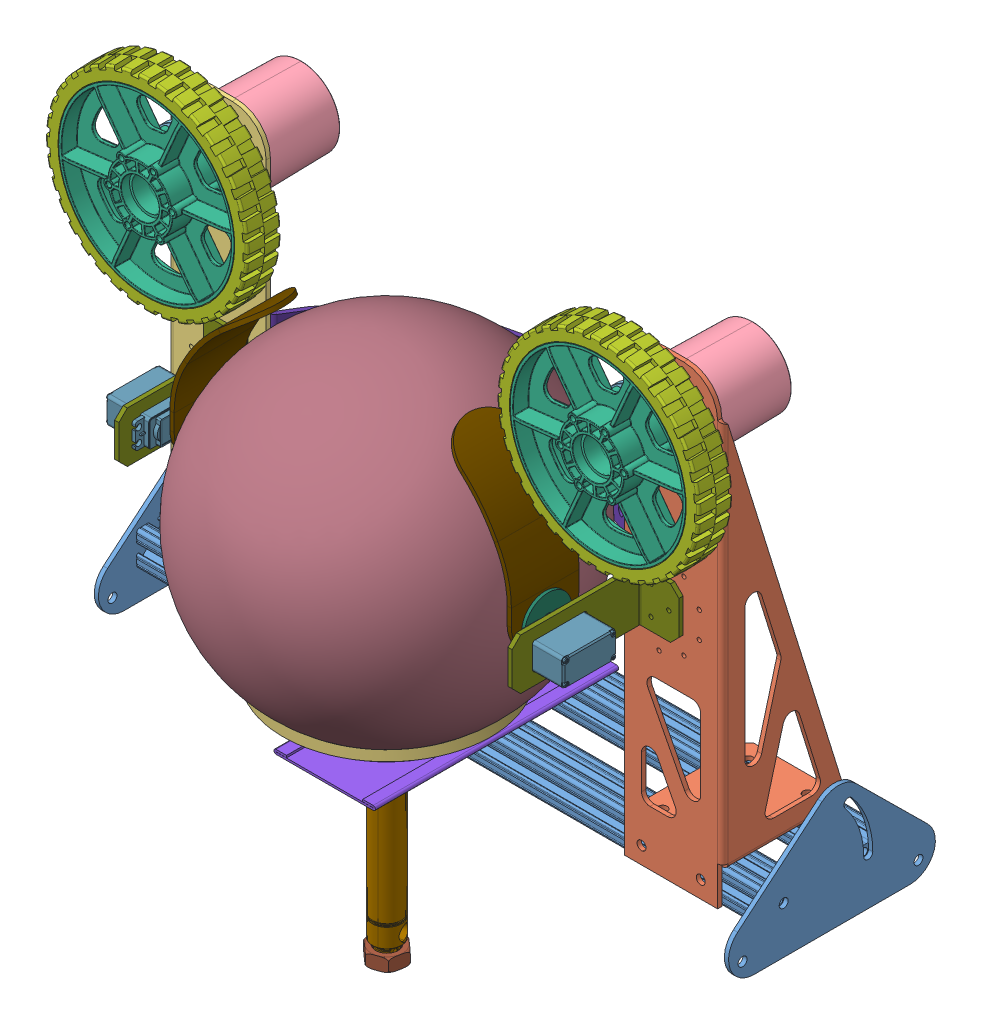
SolidWorks assembly Shooter, configuration Default. Lengths in mm.
Overall size (530.15 526.46 390.38).
32 component instances, 19 part files, 80 mates.
Components (placement in the parent):
- Shooter Base-1: Shooter Base [Default<As Machined>] at (0 35.306 -74.6762) size (469.9 25.4 88.9)
- Shooter Arm Right-1: Shooter Arm Right [Default] at (-100.3808 22.606 -61.9762) x (-1 0 0) z (0 0 -1) size (73.76 342.9 92.82)
- Shooter Arm-2: Shooter Arm [Default] at (-439.3692 22.606 -61.9762) x (-1 0 0) z (0 0 -1) size (73.76 342.9 92.82)
- REV-21-1650-1: REV-21-1650 [Default] at (-404.4442 327.406 -61.9762) x (0 1 0) z (0 0 1) size (61.14 61.02 93.25)
- REV-21-1650-2: REV-21-1650 [Default] at (-65.4558 327.406 -61.9762) x (0 1 0) z (0 0 1) size (61.14 61.02 93.25)
- am-0320a 8mm Key Hub.step-1: am-0320a 8mm Key Hub.step [Default] at (-404.4442 327.406 -33.0762) x (0.116635 -0.993175 0) z (0 0 -1) size (57.15 57.15 25.4)
- am-0320a 8mm Key Hub.step-2: am-0320a 8mm Key Hub.step [Default] at (-65.4558 327.406 -33.0762) x (0.114086 -0.993471 0) z (0 0 -1) size (57.15 57.15 25.4)
- am-0940b 6 in HiGrip Wheel-1: am-0940b 6 in HiGrip Wheel [Default] at (-424.5772 315.5538 -69.1474) x (0 0 -1) z (0.993175 0.116635 0) size (34.94 152.4 152.4)
  - 6 wheel Rev 4-1: 6 wheel Rev 4 [Default] at (-52.6446 9.4231 21.378) size (34.94 132.08 132.08)
  - 6 wheel tread II-1: 6 wheel tread II [Default] at (-65.3446 9.4231 21.378) x (0 0 -1) z (1 0 0) size (152.4 152.4 25.61)
- am-0940b 6 in HiGrip Wheel-2: am-0940b 6 in HiGrip Wheel [Default] at (-85.757 338.9677 -69.1474) x (0 0 -1) z (0.595537 -0.803328 0) size (34.94 152.4 152.4)
  - 6 wheel Rev 4-1: 6 wheel Rev 4 [Default] at (-52.6446 9.4231 21.378) size (34.94 132.08 132.08)
  - 6 wheel tread II-1: 6 wheel tread II [Default] at (-65.3446 9.4231 21.378) x (0 0 -1) z (1 0 0) size (152.4 152.4 25.61)
- Shooter Pneumatic Plate-1: Shooter Pneumatic Plate [Default] at (-196.85 49.5935 31.866) size (76.2 3.28 182.74)
- am-2034_2-1: am-2034_2 [Default] at (-234.95 -22.225 -14.9298) x (0.323379 0 0.94627) z (0 1 0) size (27.58 27.58 165.86) (flexible)
  - NCME075-0200.step_NCM-Body_075E^am-2034_2-1: NCME075-0200.step_NCM-Body_075E^am-2034_2 [Default] at origin size (21.84 21.85 153.16) (virtual)
  - NCME075-0200.step_NCM-Rod_075^am-2034_2-1: NCME075-0200.step_NCM-Rod_075^am-2034_2 [Default] at (0 0 -25.4) x (-1 0 0) z (0 0 1) size (19.05 19.05 123.53) (virtual)
  - NCME075-0200.step_NCM-Nut_075^am-2034_2-1: NCME075-0200.step_NCM-Nut_075^am-2034_2 [Default] at (0 0 77.439) x (-1 0 0) z (0 0 1) size (27.58 27.58 9.66) (virtual)
  - NCME075-0200.step_NCM-Nut_075^am-2034_2-2: NCME075-0200.step_NCM-Nut_075^am-2034_2 [Default] at (0 0 -63.119) size (27.58 27.58 9.66) (virtual)
- Shooter Cup-1: Shooter Cup [Default] at (-234.95 60.706 -14.9298) x (0.902068 0 -0.431594) z (0.431594 0 0.902068) size (155.9 37.46 155.9)
- Blue Cargo-1: Blue Cargo [Default] at (-234.95 193.4194 -14.9298) x (0.867373 -0.45742 -0.196039) z (0.420003 0.461532 0.7814) size (241.3 241.3 241.3)
- Hitec HS-325HB Korpus-3: Hitec HS-325HB Korpus [По умолчанию] at (-407.5 199.992 3.8708) x (0 0 1) z (0 1 0) size (53 41.52 20)
- Hitec HS-325HB Korpus-5: Hitec HS-325HB Korpus [По умолчанию] at (-62.4 200.82 5.0188) x (0 0 1) z (0 -1 0) size (53 41.52 20)
- Servo Horn Round-1: Servo Horn Round [Default] at (-369.3782 199.992 -6.1292) x (0 0.662146 0.749375) z (0 0.749375 -0.662146) size (35.33 5.66 35.33)
- Servo Horn Round-2: Servo Horn Round [Default] at (-100.5218 200.82 -4.9812) x (0 -0.231211 -0.972904) z (0 0.972904 -0.231211) size (35.33 5.66 35.33)
- Shooter Servo Mount-1: Shooter Servo Mount [Default] at (-84.9884 181.356 -55.6262) size (32.49 38.1 99.06)
- Shooter Servo Mount-2: Shooter Servo Mount [Default] at (-384.9116 219.456 -55.6262) x (-1 0 0) z (0 0 1) size (32.49 38.1 99.06)
- Shooter Back-1: Shooter Back [Default] at (-234.95 200.406 -65.1512) x (1 0 0) z (0 -1 0) size (403.96 84.05 76.2)
- Shooter Holders 2-1: Shooter Holders 2 [Default] at (-363.714 180.942 -31.5292) x (0 -1 0) z (0 0 1) size (125.91 60.15 53.7)
- Shooter Holders 2-2: Shooter Holders 2 [Default] at (-106.186 181.77 20.4188) x (0 -1 0) z (0 0 -1) size (125.91 60.15 53.7)
- Shooter Mount-1: Shooter Mount [Default] at (3.175 0 0) x (0 0 -1) z (1 0 0) size (215.9 98 3.17)
- Shooter Mount-2: Shooter Mount [Default] at (-469.9 0 0) x (0 0 -1) z (1 0 0) size (215.9 98 3.17)
Mates (geometry in assembly coordinates):
- Coincident7: coincident anti-aligned: plane of Shooter Base-1 through (-469.9 41.6391 -61.9762) normal (0 0 1); plane of Shooter Arm-2 through (-413.9692 340.106 -61.9762) normal (0 0 -1)
- Coincident9: coincident anti-aligned: plane of Shooter Base-1 through (-469.9 48.006 -81.0094) normal (0 1 0); plane of Shooter Arm-2 through (-439.3692 48.006 -61.9762) normal (0 -1 0)
- Coincident10: coincident anti-aligned: plane of Shooter Base-1 through (-469.9 48.006 -65.1258) normal (0 1 0); plane of Shooter Arm Right-1 through (-100.3808 48.006 -61.9762) normal (0 -1 0)
- Coincident11: coincident anti-aligned: plane of Shooter Base-1 through (-469.9 41.6391 -61.9762) normal (0 0 1); plane of Shooter Arm Right-1 through (-74.9808 340.106 -61.9762) normal (0 0 -1)
- Concentric1: concentric: cylinder of Shooter Arm-2 through (-404.4442 327.406 -58.8012) axis (0 0 -1) radius 9.0488; cylinder of Sport Planetary Gear Box-1/am-XXXX - 57 Sport 500 Hex Output Plug-1/Output Block-1 through (-279.4 242.0366 15.875) axis (0 0 -1) radius 19.05
- Coincident13: coincident: plane of Shooter Arm-2 through (-304.8 16.6116 9.525) normal (0 0 -1); plane of Sport Planetary Gear Box-1/am-XXXX - 57 Sport 500 Hex Output Plug-1/Output Block-1 through (-279.4 242.0366 9.525) normal (0 0 1)
- Parallel1: parallel aligned: plane of Shooter Arm-2 through (-413.9692 365.506 -58.8012) normal (0 1 0); plane of Sport Planetary Gear Box-1/am-XXXX - 57 Sport 1 Stage Ring Gear Housing-1 through (-303.2125 265.8491 6.35) normal (0 1 0)
- Concentric2: concentric aligned: cylinder of Shooter Arm-2 through (-404.4442 327.406 -58.8012) axis (0 0 -1) radius 9.0488; cylinder of REV-21-1650-1 through (-404.4442 327.406 -58.4762) axis (0 0 -1) radius 9.525
- Coincident15: coincident anti-aligned: plane of Shooter Arm-2 through (-413.9692 340.106 -61.9762) normal (0 0 -1); plane of REV-21-1650-1 through (-404.4442 327.406 -61.9762) normal (0 0 1)
- Parallel12: parallel aligned: plane of REV-21-1650-1 through (-404.4442 327.406 -61.9762) normal (-1 0 0); plane of Shooter Arm-2 through (-443.2808 22.606 -61.9762) normal (-1 0 0)
- Concentric3: concentric aligned: cylinder of Shooter Arm Right-1 through (-65.4558 327.406 -58.8012) axis (0 0 -1) radius 9.0488; cylinder of REV-21-1650-2 through (-65.4558 327.406 -58.4762) axis (0 0 -1) radius 9.525
- Coincident23: coincident anti-aligned: plane of Shooter Arm Right-1 through (-74.9808 340.106 -61.9762) normal (0 0 -1); plane of REV-21-1650-2 through (-65.4558 327.406 -61.9762) normal (0 0 1)
- Parallel13: parallel aligned: plane of Shooter Arm Right-1 through (-100.3808 22.606 -58.8012) normal (-1 0 0); plane of REV-21-1650-2 through (-65.4558 327.406 -61.9762) normal (-1 0 0)
- Concentric5: concentric aligned: cylinder of REV-21-1650-1 through (-404.4442 327.406 19.3375) axis (0 0 -1) radius 4; cylinder of am-0320a 8mm Key Hub.step-1 through (-404.4442 327.406 -33.0762) axis (0 0 -1) radius 4.0259
- Concentric6: concentric aligned: cylinder of REV-21-1650-2 through (-65.4558 327.406 19.3375) axis (0 0 -1) radius 4; cylinder of am-0320a 8mm Key Hub.step-2 through (-65.4558 327.406 -33.0762) axis (0 0 -1) radius 4.0259
- Concentric7: concentric anti-aligned: cylinder of REV-21-1650-1 through (-404.4442 327.406 19.3375) axis (0 0 -1) radius 4; cone of am-0940b 6 in HiGrip Wheel-1/6 wheel Rev 4-1 through (-404.4442 327.406 -16.5027) axis (0 0 1)
- Coincident25: coincident anti-aligned: plane of am-0320a 8mm Key Hub.step-1 through (-411.6956 389.1529 -33.9652) normal (0 0 1); plane of am-0940b 6 in HiGrip Wheel-1/6 wheel Rev 4-1 through (-404.4442 327.406 -33.9652) normal (0 0 -1)
- Concentric8: concentric anti-aligned: cylinder of am-0320a 8mm Key Hub.step-1 through (-380.7942 330.1834 -33.0762) axis (0 0 -1) radius 2.5908; cylinder of am-0940b 6 in HiGrip Wheel-1/6 wheel Rev 4-1 through (-380.7942 330.1834 -33.9652) axis (0 0 1) radius 1.9939
- Concentric9: concentric aligned: cylinder of am-0320a 8mm Key Hub.step-2 through (-65.4558 327.406 -33.0762) axis (0 0 -1) radius 4.0259; cone of am-0940b 6 in HiGrip Wheel-2/6 wheel Rev 4-1 through (-65.4558 327.406 -16.5027) axis (0 0 -1)
- Coincident26: coincident anti-aligned: plane of am-0320a 8mm Key Hub.step-2 through (-72.5487 389.1713 -33.9652) normal (0 0 1); plane of am-0940b 6 in HiGrip Wheel-2/6 wheel Rev 4-1 through (-65.4558 327.406 -33.9652) normal (0 0 -1)
- Concentric10: concentric anti-aligned: cylinder of am-0320a 8mm Key Hub.step-2 through (-41.7988 330.1227 -33.0762) axis (0 0 -1) radius 2.5908; cylinder of am-0940b 6 in HiGrip Wheel-2/6 wheel Rev 4-1 through (-41.7988 330.1227 -33.9652) axis (0 0 1) radius 1.9939
- Coincident27: coincident aligned: plane of am-0940b 6 in HiGrip Wheel-1/6 wheel Rev 4-1 through (-404.4442 327.406 0.9598) normal (0 0 1); plane of am-0940b 6 in HiGrip Wheel-2/6 wheel Rev 4-1 through (-65.4558 327.406 0.9598) normal (0 0 1)
- Distance5: distance = 342.9 mm aligned: plane of Shooter Arm-2 through (-369.5192 22.606 -58.8012) normal (1 0 0); plane of Shooter Arm Right-1 through (-26.6192 22.606 -61.9762) normal (1 0 0)
- Coincident32: coincident anti-aligned: plane of Shooter Base-1 through (-469.9 48.006 -144.5094) normal (0 1 0); plane of Shooter Pneumatic Plate-1 through (-196.85 48.006 31.866) normal (0 -1 0)
- Coincident33: coincident aligned: plane of Shooter Base-1 through (-469.9 44.8564 -150.8762) normal (0 0 -1); plane of Shooter Pneumatic Plate-1 through (-196.85 48.006 -150.8762) normal (0 0 -1)
- Width1: width anti-aligned: plane of Shooter Pneumatic Plate-1 through (-263.525 51.281 -59.5051) normal (1 0 0); plane of Shooter Base-1 through (-206.375 51.281 -59.5051) normal (-1 0 0); plane of Shooter Pneumatic Plate-1 through (-469.9 22.606 -132.3511) normal (-1 0 0); plane of Shooter Base-1 through (0 22.606 -68.8511) normal (1 0 0)
- Coincident34: coincident anti-aligned: plane of REV-21-1650-2 through (-65.4558 327.406 -58.4762) normal (0 0 1); plane of am-0320a 8mm Key Hub.step-2 through (-65.4558 327.406 -58.4762) normal (0 0 -1)
- Concentric11: concentric anti-aligned: cylinder of Shooter Pneumatic Plate-1 through (-234.95 48.006 -14.9298) axis (0 1 0) radius 9.525; cylinder of am-2034_2-1/am-2034_2(2)-1/NCME075-0200.step_NCM-Body_075E^am-2034_2(2)-1 through (-208.3308 -57.531 55.118) axis (0 -1 0) radius 7.9248
- Coincident35: coincident anti-aligned: plane of Shooter Pneumatic Plate-1 through (-196.85 48.006 31.866) normal (0 -1 0); plane of am-2034_2-1/am-2034_2(2)-1/NCME075-0200.step_NCM-Body_075E^am-2034_2(2)-1 through (-208.3308 12.7 55.118) normal (0 1 0)
- Parallel14: parallel anti-aligned: plane of Shooter Pneumatic Plate-1 through (-196.85 48.006 31.866) normal (0 0 1); plane of am-2034_2-1/am-2034_2(2)-1/NCME075-0200.step_NCM-Body_075E^am-2034_2(2)-1 through (-197.4088 12.7 45.593) normal (0 0 -1)
- Concentric12: concentric aligned: cylinder of am-2034_2-1/am-2034_2(2)-1/NCME075-0200.step_NCM-Rod_075^am-2034_2(2)-1 through (-208.3308 73.3837 55.118) axis (0 -1 0) radius 3.175; cylinder of Shooter Cup-1 through (-234.95 60.706 -14.9298) axis (0 -1 0) radius 2.5527
- Coincident37: coincident anti-aligned: plane of am-2034_2-1/am-2034_2(2)-1/NCME075-0200.step_NCM-Body_075E^am-2034_2(2)-1 through (-216.2683 25.4 55.118) normal (0 1 0); plane of Shooter Cup-1 through (-234.95 60.706 -14.9298) normal (0 -1 0)
- Concentric13: concentric: sphere of Shooter Cup-1; sphere of Blue Cargo-1
- Concentric14: concentric aligned: cylinder of am-2034_2-1/NCME075-0200.step_NCM-Rod_075^am-2034_2-1 through (-234.95 82.3863 -14.9298) axis (0 -1 0) radius 3.175; cylinder of Shooter Cup-1 through (-234.95 60.706 -14.9298) axis (0 -1 0) radius 2.5527
- Concentric15: concentric anti-aligned: cylinder of Shooter Pneumatic Plate-1 through (-234.95 48.006 -14.9298) axis (0 1 0) radius 9.525; cylinder of am-2034_2-1/NCME075-0200.step_NCM-Body_075E^am-2034_2-1 through (-234.95 -22.225 -14.9298) axis (0 -1 0) radius 7.9248
- Coincident38: coincident anti-aligned: plane of Shooter Pneumatic Plate-1 through (-196.85 48.006 31.866) normal (0 -1 0); plane of am-2034_2-1/NCME075-0200.step_NCM-Body_075E^am-2034_2-1 through (-234.95 48.006 -14.9298) normal (0 1 0)
- Coincident39: coincident aligned: plane of am-2034_2-1/NCME075-0200.step_NCM-Rod_075^am-2034_2-1 through (-237.9544 60.706 -13.903) normal (0 -1 0); plane of Shooter Cup-1 through (-234.95 60.706 -14.9298) normal (0 -1 0)
- Concentric16: concentric aligned: cylinder of Hitec HS-325HB Korpus-3 through (-366 199.992 -6.1292) axis (-1 0 0) radius 3; cylinder of Servo Horn Round-1 through (-369.3782 199.992 -6.1292) axis (-1 0 0) radius 2.794
- Coincident40: coincident anti-aligned: plane of Hitec HS-325HB Korpus-3 through (-366 199.992 -6.1292) normal (1 0 0); plane of Servo Horn Round-1 through (-366 201.842 -4.0355) normal (-1 0 0)
- Concentric17: concentric aligned: cylinder of Hitec HS-325HB Korpus-5 through (-103.9 200.82 -4.9812) axis (1 0 0) radius 3; cylinder of Servo Horn Round-2 through (-100.5218 200.82 -4.9812) axis (1 0 0) radius 2.794
- Coincident41: coincident anti-aligned: plane of Hitec HS-325HB Korpus-5 through (-103.9 200.82 -4.9812) normal (-1 0 0); plane of Servo Horn Round-2 through (-103.9 200.174 -7.6995) normal (1 0 0)
- Coincident42: coincident anti-aligned: plane of Servo Horn Round-2 through (-106.186 200.5087 -6.291) normal (-1 0 0); plane of Shooter Holders-2 through (-54.8526 152.814 82.395) normal (1 0 0)
- Width2: width anti-aligned: plane of Shooter Holders-2 through (-200.9026 178.214 66.52) normal (0 1 0); plane of Shooter Holders-2 through (-200.9026 152.814 66.52) normal (0 -1 0); plane of Hitec HS-325HB Korpus-5 through (-94.9 190.82 -12.9812) normal (0 -1 0); plane of Hitec HS-325HB Korpus-5 through (-94.9 210.82 -12.9812) normal (0 1 0)
- Parallel15: parallel aligned: plane of Shooter Pneumatic Plate-1 through (-196.85 49.5935 31.866) normal (0 1 0); plane of Hitec HS-325HB Korpus-5 through (-94.9 210.82 -12.9812) normal (0 1 0)
- Coincident46: coincident anti-aligned: plane of Shooter Arm Right-1 through (-76.9366 91.5119 177.0821) normal (-1 0 0); plane of Hitec HS-325HB Korpus-5 through (-65.4558 266.7892 103.8097) normal (1 0 0)
- Coincident47: coincident anti-aligned: plane of Hitec HS-325HB Korpus-5 through (-94.9 192.82 25.0188) normal (0 0 1); plane of Shooter Servo Mount-1 through (-56.4124 192.532 25.0188) normal (0 0 -1)
- Coincident48: coincident anti-aligned: plane of Hitec HS-325HB Korpus-5 through (-94.9 210.82 -12.9812) normal (0 1 0); plane of Shooter Servo Mount-1 through (-56.4124 210.82 -13.5892) normal (0 -1 0)
- Coincident49: coincident anti-aligned: plane of Hitec HS-325HB Korpus-5 through (-88.9 208.5084 -19.6696) normal (1 0 0); plane of Shooter Servo Mount-1 through (-88.9 181.356 -55.6262) normal (-1 0 0)
- Coincident50: coincident anti-aligned: plane of Shooter Arm Right-1 through (-74.9808 340.106 -58.8012) normal (0 0 1); plane of Shooter Servo Mount-1 through (-84.9884 181.356 -58.8012) normal (0 0 -1)
- Coincident52: coincident aligned: plane of Shooter Servo Mount-1 through (-88.9 219.456 -55.6262) normal (0 1 0); plane of Shooter Servo Mount-2 through (-381 219.456 40.2588) normal (0 1 0)
- Coincident53: coincident anti-aligned: plane of Hitec HS-325HB Korpus-3 through (-375 189.992 -14.1292) normal (0 -1 0); plane of Shooter Servo Mount-2 through (-413.4876 189.992 -13.5892) normal (0 1 0)
- Coincident54: coincident anti-aligned: plane of Hitec HS-325HB Korpus-3 through (-375 207.992 -16.1292) normal (0 0 -1); plane of Shooter Servo Mount-2 through (-413.4876 208.28 -16.1292) normal (0 0 1)
- Coincident55: coincident anti-aligned: plane of Hitec HS-325HB Korpus-3 through (-381 192.3036 -20.8176) normal (-1 0 0); plane of Shooter Servo Mount-2 through (-381 219.456 -55.6262) normal (1 0 0)
- Coincident56: coincident anti-aligned: plane of Shooter Arm-2 through (-413.9692 340.106 -58.8012) normal (0 0 1); plane of Shooter Servo Mount-2 through (-384.9116 219.456 -58.8012) normal (0 0 -1)
- Concentric19: concentric aligned: cylinder of Servo Horn Round-2 through (-100.5218 200.82 -4.9812) axis (1 0 0) radius 1.3462; cylinder of Shooter Holders-2 through (-56.4401 165.514 69.695) axis (1 0 0) radius 3.3782
- Distance9: distance = 158.75 mm aligned: plane of Shooter Servo Mount-2 through (-384.9116 181.356 -58.8012) normal (0 -1 0); plane of Shooter Arm-2 through (-439.3692 22.606 -58.8012) normal (0 -1 0)
- Coincident59: coincident anti-aligned: plane of Shooter Arm Right-1 through (-74.9808 340.106 -61.9762) normal (0 0 -1); plane of Shooter Back-1 through (-32.9692 162.306 -61.9762) normal (0 0 1)
- Width4: width aligned: plane of Shooter Back-1 through (-436.9308 162.306 -65.1512) normal (-1 0 0); plane of Shooter Arm Right-1 through (-32.9692 162.306 -61.9762) normal (1 0 0); plane of Shooter Back-1 through (-29.7942 22.606 -61.9762) normal (-1 0 0); plane of Shooter Arm-2 through (-440.1058 22.606 -61.9762) normal (1 0 0)
- Width5: width aligned: plane of Shooter Back-1 through (-103.3875 238.506 -64.0419) normal (0 1 0); plane of Shooter Servo Mount-1 through (-369.9611 162.306 -65.8878) normal (0 -1 0); plane of Shooter Back-1 through (-88.9 219.456 -55.6262) normal (0 1 0); plane of Shooter Servo Mount-1 through (-88.9 181.356 40.2588) normal (0 -1 0)
- Coincident62: coincident anti-aligned: plane of Servo Horn Round-1 through (-363.714 200.8834 -5.1204) normal (1 0 0); plane of Shooter Holders 2-1 through (-363.714 180.942 19.2708) normal (-1 0 0)
- Concentric20: concentric anti-aligned: cylinder of Servo Horn Round-1 through (-369.3782 199.992 -6.1292) axis (-1 0 0) radius 1.3462; cylinder of Shooter Holders 2-1 through (-363.714 199.992 -6.1292) axis (1 0 0) radius 1.5875
- Distance12: distance = 292.1 mm anti-aligned: plane of Shooter Servo Mount-2 through (-381 219.456 -55.6262) normal (1 0 0); plane of Shooter Servo Mount-1 through (-88.9 181.356 -55.6262) normal (-1 0 0)
- Width7: width anti-aligned: plane of Shooter Servo Mount-2 through (-413.4866 219.456 -58.8012) normal (-1 0 0); plane of Shooter Arm Right-1 through (-56.4134 181.356 -58.8012) normal (1 0 0); plane of Shooter Servo Mount-1 through (-26.6192 22.606 -61.9762) normal (1 0 0); plane of Shooter Arm-2 through (-443.2808 22.606 -61.9762) normal (-1 0 0)
- Coincident66: coincident anti-aligned: plane of Servo Horn Round-2 through (-106.186 200.5087 -6.291) normal (-1 0 0); plane of Shooter Holders 2-2 through (-106.186 181.77 -30.3812) normal (1 0 0)
- Concentric21: concentric anti-aligned: cylinder of Servo Horn Round-2 through (-100.5218 200.82 -4.9812) axis (1 0 0) radius 1.3462; cylinder of Shooter Holders 2-2 through (-106.186 200.82 -4.9812) axis (-1 0 0) radius 1.5875
- Parallel16: parallel aligned: plane of Shooter Holders 2-1 through (-248.311 201.7818 19.2708) normal (0 0 1); plane of Shooter Holders 2-2 through (-119.211 256.5037 20.4188) normal (0 0 1)
- Parallel17: parallel aligned: plane of Shooter Servo Mount-1 through (-88.9 219.456 40.2588) normal (0 0 1); plane of Shooter Holders 2-2 through (-119.211 256.5037 20.4188) normal (0 0 1)
- Coincident70: coincident aligned: plane of Shooter Mount-1 through (0 0 -52.3394) normal (0 -1 0); plane of Shooter Mount-2 through (-473.075 0 -52.3394) normal (0 -1 0)
- Coincident71: coincident anti-aligned: plane of Shooter Mount-2 through (-473.075 0 -52.3394) normal (0 -1 0)
- Coincident72: coincident anti-aligned: plane of Shooter Mount-1 through (0 19.05 -52.3394) normal (-1 0 0)
- Coincident74: coincident anti-aligned: plane of Shooter Mount-1 through (3.175 0 0) normal (0 0 -1)
- Concentric22: concentric aligned: cylinder of Shooter Mount-1 through (0 12.7 -175.8884) axis (1 0 0) radius 3.3782; cylinder of Shooter Mount-2 through (-473.075 12.7 -175.8884) axis (1 0 0) radius 3.3782
- Parallel18: parallel anti-aligned: plane of Shooter Mount-1 through (0 19.05 -52.3394) normal (-1 0 0); plane of Shooter Mount-2 through (-469.9 19.05 -52.3394) normal (1 0 0)
- Coincident76: coincident anti-aligned: plane of Shooter Base-1 through (0 22.606 -132.3511) normal (1 0 0); plane of Shooter Mount-1 through (0 19.05 -52.3394) normal (-1 0 0)
- Coincident77: coincident anti-aligned: plane of Shooter Base-1 through (-469.9 22.606 -132.3511) normal (-1 0 0); plane of Shooter Mount-2 through (-469.9 19.05 -52.3394) normal (1 0 0)
- Concentric23: concentric aligned: cylinder of Shooter Base-1 through (-469.9 35.306 -74.6762) axis (1 0 0) radius 2.6035; cylinder of Shooter Mount-2 through (-473.075 35.306 -74.6762) axis (1 0 0) radius 3.3782
- Concentric24: concentric aligned: cylinder of Shooter Base-1 through (-469.9 35.306 -74.6762) axis (1 0 0) radius 2.6035; cylinder of Shooter Mount-1 through (0 35.306 -74.6762) axis (1 0 0) radius 3.3782
- Slot1: slot aligned: cylinder of Shooter Base-1 through (-469.9 35.306 -138.1762) axis (1 0 0) radius 2.6035; cylinder of Shooter Mount-1 through (0 35.306 -138.1762) axis (1 0 0) radius 3.3782; cylinder of Shooter Mount-1 through (0 35.306 -138.1762) axis (1 0 0) radius 3.3782
- Slot2: slot aligned: cylinder of Shooter Base-1 through (-469.9 35.306 -138.1762) axis (1 0 0) radius 2.6035; cylinder of Shooter Mount-2 through (-473.075 35.306 -138.1762) axis (1 0 0) radius 3.3782; cylinder of Shooter Mount-2 through (-473.075 35.306 -138.1762) axis (1 0 0) radius 3.3782
- Width8: width anti-aligned: plane of Shooter Arm-2 through (-443.2808 22.606 -61.9762) normal (-1 0 0); plane of Shooter Arm Right-1 through (-26.6192 22.606 -61.9762) normal (1 0 0); plane of Shooter Base-1 through (0 22.606 -68.8511) normal (1 0 0); plane of Shooter Base-1 through (-469.9 22.606 -68.8511) normal (-1 0 0)
